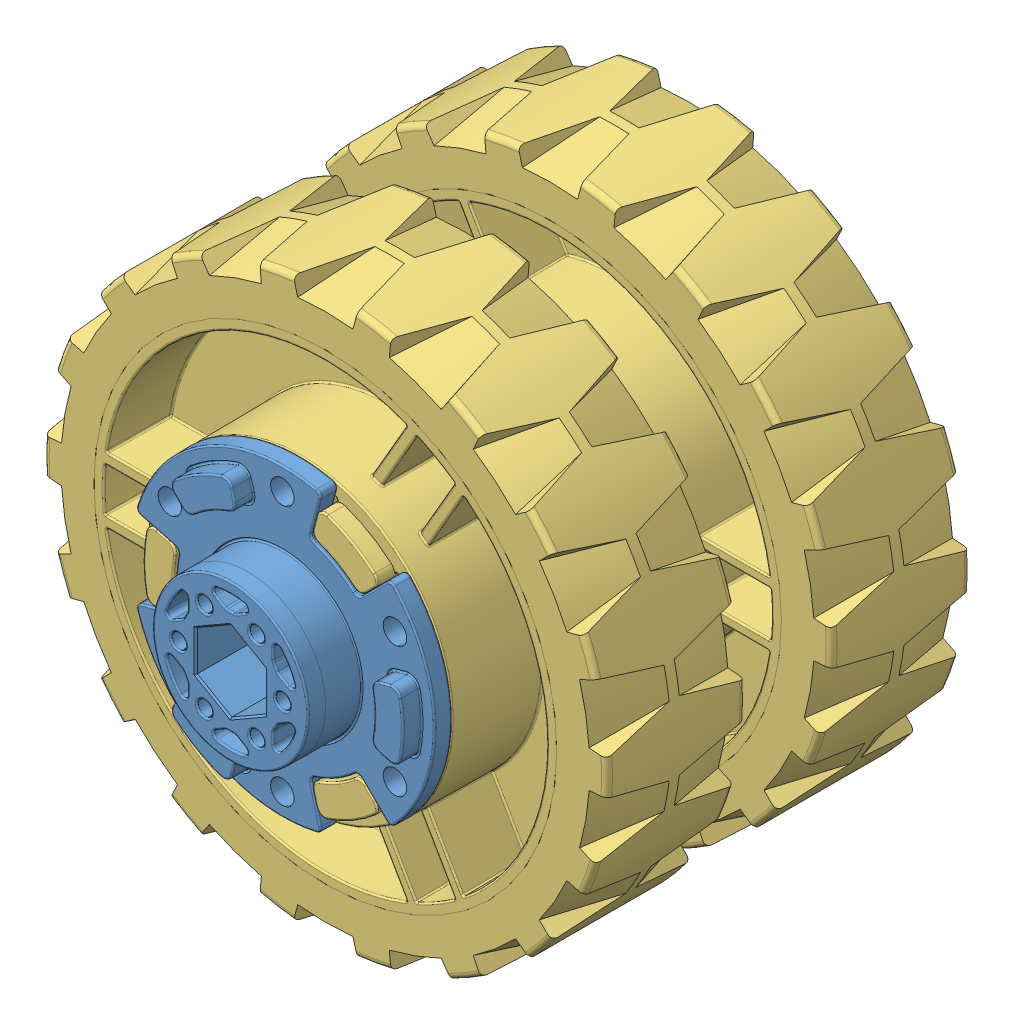
SolidWorks assembly 0001 - 03 - 1030 WHEEL ASSEMBLY, configuration Default. Lengths in mm.
Overall size (140.96 140.96 101.35).
5 component instances, 3 part files, 12 mates.
Components (placement in the parent):
- VersaHub-1: VersaHub [Default] at (4.8265 26.3593 48.1847) size (54.75 55.87 12.7)
- VersaThing-1: VersaThing [Default] at (4.8265 26.3593 8.6242) x (-0.5 0.866025 0) z (0.866025 0.5 0) size (55.88 12.7 55.88)
- VEX Wheel 4in DT-1: VEX Wheel 4in DT [Default] at (4.8265 26.3593 29.1982) x (0.5 -0.866025 0) z (0 0 1) size (103.19 103.19 41.15)
- VersaHub-2: VersaHub [Default] at (4.8265 26.3593 -30.9363) x (-0.5 -0.866025 0) z (0 0 -1) size (54.75 55.87 12.7)
- VEX Wheel 4in DT-2: VEX Wheel 4in DT [Default] at (4.8265 26.3593 -11.9498) size (103.19 103.19 41.15)
Mates (geometry in assembly coordinates):
- Concentric1: concentric aligned: cone of VersaHub-1 through (4.8265 26.3593 46.9024) axis (0 0 1); cone of VEX Wheel 4in DT-1 through (4.8265 26.3593 30.4955) axis (0 0 1)
- Concentric2: concentric anti-aligned: cylinder of VersaHub-1 through (25.4487 38.2655 46.5972) axis (0 0 1) radius 2.1526; cylinder of VEX Wheel 4in DT-1 through (25.4487 38.2655 18.1809) axis (0 0 -1) radius 2.1526
- Coincident1: coincident anti-aligned: plane of VersaHub-1 through (4.8265 26.3593 46.5972) normal (0 0 -1); plane of VEX Wheel 4in DT-1 through (4.8265 26.3593 46.5972) normal (0 0 1)
- Coincident2: coincident anti-aligned: plane of VersaThing-1 through (4.8265 26.3593 11.7992) normal (0 0 1); plane of VEX Wheel 4in DT-1 through (4.8265 26.3593 11.7992) normal (0 0 -1)
- Concentric3: concentric aligned: cylinder of VersaThing-1 through (4.8265 26.3593 5.4492) axis (0 0 1) radius 14.3; cylinder of VEX Wheel 4in DT-1 through (4.8265 26.3593 11.7992) axis (0 0 1) radius 14.3
- Concentric4: concentric aligned: cylinder of VersaThing-1 through (4.8265 50.1718 8.6242) axis (0 0 -1) radius 2.1526; cylinder of VEX Wheel 4in DT-1 through (4.8265 50.1718 18.1809) axis (0 0 -1) radius 2.1526
- Concentric5: concentric anti-aligned: cone of VEX Wheel 4in DT-1 through (4.8265 26.3593 27.9008) axis (0 0 -1); cone of VEX Wheel 4in DT-2 through (4.8265 26.3593 -10.6525) axis (0 0 1)
- Concentric6: concentric aligned: cylinder of VersaThing-1 through (4.8265 50.1718 8.6242) axis (0 0 -1) radius 2.1526; cylinder of VEX Wheel 4in DT-2 through (4.8265 50.1718 -22.9671) axis (0 0 -1) radius 2.1526
- Coincident5: coincident anti-aligned: plane of VersaThing-1 through (4.8265 26.3593 5.4492) normal (0 0 -1); plane of VEX Wheel 4in DT-2 through (4.8265 26.3593 5.4492) normal (0 0 1)
- Coincident6: coincident: plane of VersaHub-2 through (4.8265 26.3593 -29.3488) normal (0 0 1); plane of VEX Wheel 4in DT-2 through (4.8265 26.3593 -29.3488) normal (0 0 -1)
- Concentric7: concentric: cylinder of VersaHub-2 through (4.8265 26.3593 -42.0488) axis (0 0 1) radius 14.3002; cylinder of VEX Wheel 4in DT-2 through (4.8265 26.3593 -29.3488) axis (0 0 1) radius 14.3
- Concentric8: concentric aligned: cylinder of VersaHub-2 through (4.8265 50.1718 -29.3488) axis (0 0 -1) radius 2.1526; cylinder of VEX Wheel 4in DT-2 through (4.8265 50.1718 -22.9671) axis (0 0 -1) radius 2.1526
